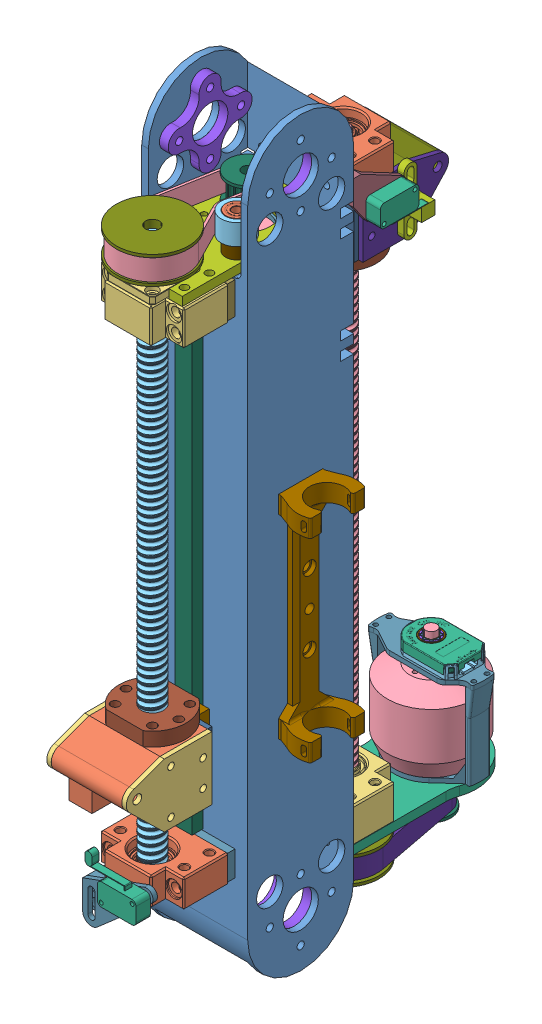
SolidWorks assembly Shoulder, configuration Default. Lengths in mm.
Overall size (114.36 533.4 280.38).
87 component instances, 45 part files, 83 mates.
Components (placement in the parent):
- Box-1: Box [Round] at origin size (76.2 533.4 76.2)
- BF12-1: BF12 [Default] at (0 614.1315 -46.7041) x (1 0 0) z (0 1 0) size (60 43 20)
- BK12-1: BK12 [Default] at (0 212.1315 -46.7041) x (-1 0 0) z (0 -1 0) size (60 46.94 35.34)
- SFU1605-450-1: SFU1605-450 [1605-400] at (0 171.1315 -71.7041) x (1 0 0) z (0 -1 0) size (16.52 16.22 450)
- BK12-2: BK12 [Default] at (0 582.269 40.2909) x (-1 0 0) z (0 1 0) size (60 46.94 35.34)
- BF12-2: BF12 [Default] at (0 230.269 40.2909) x (-1 0 0) z (0 1 0) size (60 43 20)
- SFU1605-400-3: SFU1605-400 [1605-400] at (0 623.269 65.2909) x (-1 0 0) z (0 1 0) size (16.52 16.22 400)
- J3Plate^Shoulder-1: J3Plate^Shoulder [Default] at origin size (65 6.35 120.35) (virtual)
- J2Plate^Shoulder-1: J2Plate^Shoulder [Default] at origin size (65 6.35 107.35) (virtual)
- J3MGN12R-1: J3MGN12R [Default] at origin size (12 379.5 8)
- J3MGN12C-1: J3MGN12C [Default] at (0 580.7871 -49.3066) x (1 0 0) z (0 1 0) size (27 10 45.5)
- CarriagePlate^Shoulder-1: CarriagePlate^Shoulder [Default] at (0 214.8102 -3.2066) size (50.8 45.5 3.17) (virtual)
- nut-1: nut [Default] at (0 558.0371 -71.7041) x (-1 0 0) z (0 -1 0) size (48 40 42)
- BKSpacer^Shoulder-1: BKSpacer^Shoulder [Default] at origin size (58 23 8.6) (virtual)
- BKSpacer^Shoulder-2: BKSpacer^Shoulder [Default] at (0 370.1375 81.5975) size (58 23 8.6) (virtual)
- BFSpacer^Shoulder-1: BFSpacer^Shoulder [Default] at origin size (67.1 32.07 40.22) (virtual)
- BFSpacerWSwitchMount^Shoulder-1: BFSpacerWSwitchMount^Shoulder [Default] at (0 -383.8625 81.5975) size (58 48.16 51.57) (virtual)
- J2MGN12R^Shoulder-1: J2MGN12R^Shoulder [Default] at origin size (12 329.5 8) (virtual)
- J3Adapter^Shoulder-2: J3Adapter^Shoulder [Default] at (0 224.1764 -3.2066) size (57.15 45.5 61.61) (virtual)
  - Body^J3Adapter_Shoulder-1: Body^J3Adapter_Shoulder [Default] at (38.1 26.927 0) x (0 0 -1) z (1 0 0) size (61.61 45.5 50.8) (virtual)
  - SidePlate^J3Adapter_Shoulder-1: SidePlate^J3Adapter_Shoulder [Default] at origin size (3.18 45.5 61.61) (virtual)
  - SidePlate^J3Adapter_Shoulder-2: SidePlate^J3Adapter_Shoulder [Default] at (53.975 0 0) size (3.18 45.5 61.61) (virtual)
  - 94459A340_BRASS HEAT-SET INSERT FOR PLASTIC-1: 94459A340_BRASS HEAT-SET INSERT FOR PLASTIC [94459A340] at (-18.415 340.7357 -83.735) x (0 -1 0) z (0 0 -1) size (7.22 6.55 7.22)
  - 94459A180_BRASS HEAT-SET INSERT FOR PLASTIC-1: 94459A180_BRASS HEAT-SET INSERT FOR PLASTIC [94459A180] at (13.435 343.3607 -81.9325) x (-0.837169 0 -0.546944) z (-0.546944 0 0.837169) size (7.17 9.73 7.17)
- J3MGN12C-2: J3MGN12C [Default] at (0 297.5146 42.8934) x (-1 0 0) z (0 1 0) size (27 10 45.5)
- nut-2: nut [Default] at (0 320.2646 65.2909) x (1 0 0) z (0 1 0) size (48 40 42)
- J2Adapter^Shoulder-1: J2Adapter^Shoulder [Default] at (0 654.1252 -3.2066) x (1 0 0) z (0 0 -1) size (57.15 45.5 61.61) (virtual)
  - Body^J2Adapter_Shoulder-1: Body^J2Adapter_Shoulder [Default] at (38.1 26.927 0) x (0 0 -1) z (1 0 0) size (61.61 45.5 50.8) (virtual)
  - SidePlate1fix-1: SidePlate1fix [Default] at origin size (3.18 45.5 61.61)
  - SidePlate1fix-2: SidePlate1fix [Default] at (53.975 0 0) size (3.18 45.5 61.61)
  - 94459A340_BRASS HEAT-SET INSERT FOR PLASTIC-1: 94459A340_BRASS HEAT-SET INSERT FOR PLASTIC [94459A340] at (-18.415 340.7357 -83.735) x (0 -1 0) z (0 0 -1) size (7.22 6.55 7.22)
  - 94459A180_BRASS HEAT-SET INSERT FOR PLASTIC-1: 94459A180_BRASS HEAT-SET INSERT FOR PLASTIC [94459A180] at (13.435 343.3607 -81.9325) x (-0.837169 0 -0.546944) z (-0.546944 0 0.837169) size (7.17 9.73 7.17)
- CarriagePlate^Shoulder-2: CarriagePlate^Shoulder [Default] at (0 -68.4623 -3.2066) x (-1 0 0) z (0 0 -1) size (50.8 45.5 3.17) (virtual)
- 192kvMotorEncoded-1: 192kvMotorEncoded [Default] at (0 202.8065 -135.2041) x (0 0 -1) z (1 0 0) size (63 104.52 76.93)
  - BetterKEDA-1: BetterKEDA [Default] at origin size (63 104.52 63)
  - CUI_DEVICES_AMT102-0048-N2000-S-1: CUI_DEVICES_AMT102-0048-N2000-S [Default] at (0 65.12 0) x (1 0 0) z (0 1 0) size (36.33 46.21 9.2)
    - CUI_DEVICES_AMT102-0048-N2000-S.step-1: CUI_DEVICES_AMT102-0048-N2000-S.step [Default] at origin size (36.33 46.21 9.2)
      - AMT-102-Base-REV-K.step-1: AMT-102-Base-REV-K.step [Default] x (-1 0 0) z (0 0 -1) size (28.78 43.39 9.06)
      - AMT-102-Top-Cover-REV-H.step-1: AMT-102-Top-Cover-REV-H.step [Default] at (0 0 5.23) x (-1 0 0) z (0 0 -1) size (28.6 43.26 6.55)
      - AMT-Sleeve-REV-D_ 2 mm.step-1: AMT-Sleeve-REV-D_ 2 mm.step [Default] at (0 0 -2.42) x (0.999996 0.002864 0) z (0 0 1) size (10.79 10.79 7.8)
      - AMT-Hub-Top-REV-D1.step-1: AMT-Hub-Top-REV-D1.step [Default] at (0 0 2.13) x (0.999996 0.002864 0) z (0 0 1) size (14 14 5.67)
      - AMT-Hub-Bottom-REV-B.step-1: AMT-Hub-Bottom-REV-B.step [Default] at (0 0 2.43) x (0.999998 -0.001942 0) z (0 0 1) size (17.3 17.3 3.2)
      - AMT10X-Shaft-Adaptor-REV-E.step-1: AMT10X-Shaft-Adaptor-REV-E.step [Default] at (0 0 0.03) x (0.999996 0.002864 0) z (0 0 1) size (11.8 11.8 7.8)
      - Receiver-board.step-1: Receiver-board.step [Default] at (72.2834 -20.351 3.03) x (-1 0 0) z (0 0 -1) size (26.5 26.62 0.41)
      - Rotor-board-REV F.step-1: Rotor-board-REV F.step [Default] at (0 0 2.13) x (0.807874 -0.589355 0) z (0 0 1) size (26 26 0.3)
      - Transmitter-board AMT10_AMT-102.step-1: Transmitter-board AMT10_AMT-102.step [Default] at (19.1596 -17.1102 1.22) x (-1 0 0) z (0 0 -1) size (26.63 38.43 4.41)
  - Body^192kvMotorEncoded-1: Body^192kvMotorEncoded [Default] at origin size (53 64.53 76.93) (virtual)
- 192kvMotorEncoded-2: 192kvMotorEncoded [Default] at (0 591.594 -3.2066) x (-0.707107 0 -0.707107) z (-0.707107 0 0.707107) size (63 104.52 76.93)
  - BetterKEDA-1: BetterKEDA [Default] at origin size (63 104.52 63)
  - CUI_DEVICES_AMT102-0048-N2000-S-1: CUI_DEVICES_AMT102-0048-N2000-S [Default] at (0 65.12 0) x (1 0 0) z (0 1 0) size (36.33 46.21 9.2)
    - CUI_DEVICES_AMT102-0048-N2000-S.step-1: CUI_DEVICES_AMT102-0048-N2000-S.step [Default] at origin size (36.33 46.21 9.2)
      - AMT-102-Base-REV-K.step-1: AMT-102-Base-REV-K.step [Default] x (-1 0 0) z (0 0 -1) size (28.78 43.39 9.06)
      - AMT-102-Top-Cover-REV-H.step-1: AMT-102-Top-Cover-REV-H.step [Default] at (0 0 5.23) x (-1 0 0) z (0 0 -1) size (28.6 43.26 6.55)
      - AMT-Sleeve-REV-D_ 2 mm.step-1: AMT-Sleeve-REV-D_ 2 mm.step [Default] at (0 0 -2.42) x (0.999996 0.002864 0) z (0 0 1) size (10.79 10.79 7.8)
      - AMT-Hub-Top-REV-D1.step-1: AMT-Hub-Top-REV-D1.step [Default] at (0 0 2.13) x (0.999996 0.002864 0) z (0 0 1) size (14 14 5.67)
      - AMT-Hub-Bottom-REV-B.step-1: AMT-Hub-Bottom-REV-B.step [Default] at (0 0 2.43) x (0.999998 -0.001942 0) z (0 0 1) size (17.3 17.3 3.2)
      - AMT10X-Shaft-Adaptor-REV-E.step-1: AMT10X-Shaft-Adaptor-REV-E.step [Default] at (0 0 0.03) x (0.999996 0.002864 0) z (0 0 1) size (11.8 11.8 7.8)
      - Receiver-board.step-1: Receiver-board.step [Default] at (72.2834 -20.351 3.03) x (-1 0 0) z (0 0 -1) size (26.5 26.62 0.41)
      - Rotor-board-REV F.step-1: Rotor-board-REV F.step [Default] at (0 0 2.13) x (0.807874 -0.589355 0) z (0 0 1) size (26 26 0.3)
      - Transmitter-board AMT10_AMT-102.step-1: Transmitter-board AMT10_AMT-102.step [Default] at (19.1596 -17.1102 1.22) x (-1 0 0) z (0 0 -1) size (26.63 38.43 4.41)
  - Body^192kvMotorEncoded-1: Body^192kvMotorEncoded [Default] at origin size (53 64.53 76.93) (virtual)
- 15Tpulley-3: 15Tpulley [Default] at (0 175.8815 -135.2041) size (28 28 28)
- 15Tpulley-4: 15Tpulley [Default] at (0 618.519 -3.2066) x (-1 0 0) z (0 0 1) size (28 28 28)
- 30Tpulley-3: 30Tpulley [Default] at (0 618.519 65.2909) size (52 20 52)
- 30Tpulley-4: 30Tpulley [Default] at (0 175.8815 -71.7041) size (52 20 52)
- J3Belt51T^Shoulder-1: J3Belt51T^Shoulder [Default] at origin size (49.49 15 101.05) (virtual)
- TensionPillarJ3-1: TensionPillarJ3 [Default] at (-42.5291 257.8915 3.8215) size (33.31 25.73 33.31)
  - 92510A774_ALUM UNTHRD SPACER-1-1: 92510A774_ALUM UNTHRD SPACER-1 [92510A774] at (20.3041 -69.3725 -110.4505) x (1 0 0) z (0 1 0) size (15.88 15.88 9.53)
  - 98019A228_MIL SPEC. 300 SERIES SS FLAT WASHER-1: 98019A228_MIL SPEC. 300 SERIES SS FLAT WASHER [98019A228] at (20.3041 -74.8462 -110.4505) x (0.972939 0 -0.231063) z (0.231063 0 0.972939) size (9.53 0.71 9.53)
  - 60355K701_BALL BEARING-1: 60355K701_BALL BEARING [60355K701] at (20.3041 -77.3354 -110.4505) x (1 0 0) z (0 1 0) size (15.88 15.88 4.98)
  - Roller^TensionPillarJ3-1: Roller^TensionPillarJ3 [Default] at (-2.0675 -22.8548 2.6827) size (33.31 15 33.31) (virtual)
  - 60355K701_BALL BEARING-2: 60355K701_BALL BEARING [60355K701] at (20.3041 -87.8548 -110.4505) x (1 0 0) z (0 1 0) size (15.88 15.88 4.98)
- J2Belt52T^Shoulder-1: J2Belt52T^Shoulder [Default] at origin size (49.49 15 106.05) (virtual)
- TensionPillarJ2-1: TensionPillarJ2 [Default] at (19.05 605.8815 23.7809) x (-1 0 0) z (0 1 0) size (22.23 22.23 25.73)
  - 92510A774_ALUM UNTHRD SPACER-1-1: 92510A774_ALUM UNTHRD SPACER-1 [92510A774] x (1 0 0) z (0 0 -1) size (15.88 15.88 9.53)
  - 98019A228_MIL SPEC. 300 SERIES SS FLAT WASHER-1: 98019A228_MIL SPEC. 300 SERIES SS FLAT WASHER [98019A228] at (0 0 5.4737) x (0.972939 -0.231063 0) z (0.231063 0.972939 0) size (9.53 0.71 9.53)
  - 60355K701_BALL BEARING-1: 60355K701_BALL BEARING [60355K701] at (0 0 7.9629) x (1 0 0) z (0 0 -1) size (15.88 15.88 4.98)
  - Roller^TensionPillarJ2-1: Roller^TensionPillarJ2 [Default] at (-22.3716 113.1333 -52.2073) x (1 0 0) z (0 1 0) size (22.23 15 22.23) (virtual)
  - 60355K701_BALL BEARING-2: 60355K701_BALL BEARING [60355K701] at (0 0 18.4823) x (1 0 0) z (0 0 -1) size (15.88 15.88 4.98)
- switch-1: switch [Default] at (43.25 594.2315 -52.9416) x (0 0 1) z (0 1 0) size (39.3 10.3 27.5)
- Trigger^Shoulder-1: Trigger^Shoulder [Default] at (-1.6066 -39.0023 -12.3199) size (17.46 47.62 9.53) (virtual)
- switch-2: switch [Default] at (16.85 229.869 91.6159) x (1 0 0) z (0 -1 0) size (39.3 10.3 27.5)
- ShaftSupp^Shoulder-1: ShaftSupp^Shoulder [Default] at origin size (6.35 60.32 60.32)
- ShaftSupp^Shoulder-2: ShaftSupp^Shoulder [Default] at (0 457.2 0) size (6.35 60.32 60.32)
- ShaftSupp^Shoulder-5: ShaftSupp^Shoulder [Default] at (0 0 -6.4131) x (-1 0 0) z (0 0 -1) size (6.35 60.32 60.32)
- ShaftSupp^Shoulder-6: ShaftSupp^Shoulder [Default] at (0 457.2 -6.4131) x (-1 0 0) z (0 0 -1) size (6.35 60.32 60.32)
- WireGuide^Shoulder-1: WireGuide^Shoulder [Default] at origin size (26.79 152.4 42.24) (virtual)
Mates (geometry in assembly coordinates):
- Parallel1: parallel anti-aligned: plane of Box-1 through (-33.3375 186.9315 -41.3066) normal (0 0 -1); plane of BF12-1 through (29 605.1315 -46.7041) normal (0 0 1)
- Width1: width anti-aligned: plane of BF12-1 through (30 605.1315 -78.2041) normal (1 0 0); plane of BF12-1 through (-30 605.1315 -47.7041) normal (-1 0 0); plane of Box-1 through (38.1 644.1315 -3.2066) normal (1 0 0); plane of Box-1 through (-38.1 186.9315 -3.2066) normal (-1 0 0)
- Distance6: distance anti-aligned: plane of Box-1 through (-33.3375 186.9315 -41.3066) normal (0 0 -1); plane of BK12-1 through (-29 223.6315 -46.7041) normal (0 0 1)
- Width2: width aligned: plane of BK12-1 through (30 223.6315 -47.7041) normal (1 0 0); plane of BK12-1 through (-30 223.6315 -78.2041) normal (-1 0 0); plane of Box-1 through (-38.1 186.9315 -3.2066) normal (-1 0 0); plane of Box-1 through (38.1 644.1315 -3.2066) normal (1 0 0)
- Parallel3: parallel aligned: plane of BK12-1 through (29 224.6315 -47.7041) normal (0 1 0)
- Coincident11: coincident: line of SFU1605-450-1 through (0 185.8815 -71.7041) axis (0 -1 0)
- Concentric6: concentric anti-aligned: cylinder of BK12-1 through (0 220.1315 -71.7041) axis (0 1 0) radius 6; cylinder of SFU1605-450-1 through (0 186.1315 -71.7041) axis (0 -1 0) radius 5
- Coincident12: coincident anti-aligned: plane of BK12-1 through (7.2358 225.1315 -64.4683) normal (0 1 0); plane of SFU1605-450-1 through (0 225.1315 -71.7041) normal (0 -1 0)
- Coincident13: coincident anti-aligned: plane of BF12-1 through (-6.5021 610.1315 -65.202) normal (0 -1 0); plane of SFU1605-450-1 through (0 610.1315 -71.7041) normal (0 1 0)
- Distance3: distance = 12.7 mm: plane of BK12-1 through (29 199.6315 -47.7041) normal (0 -1 0); line of Box-1 through (38.1 186.9315 -41.3066) axis (-1 0 0)
- Coincident27: coincident: line of SFU1605-400-3 through (0 608.519 65.2909) axis (0 1 0)
- Concentric18: concentric anti-aligned: cylinder of BK12-2 through (0 582.269 65.2909) axis (0 -1 0) radius 6; cylinder of SFU1605-400-3 through (0 608.269 65.2909) axis (0 1 0) radius 5
- Distance8: distance anti-aligned: plane of Box-1 through (-33.3375 186.9315 34.8934) normal (0 0 1); plane of BK12-2 through (-29 570.769 40.2909) normal (0 0 -1)
- Coincident29: coincident anti-aligned: plane of BK12-2 through (7.2358 569.269 58.0551) normal (0 -1 0); plane of SFU1605-400-3 through (0 569.269 65.2909) normal (0 1 0)
- Coincident30: coincident anti-aligned: plane of BF12-2 through (-6.5021 234.269 58.7888) normal (0 1 0); plane of SFU1605-400-3 through (0 234.269 65.2909) normal (0 -1 0)
- Concentric19: concentric anti-aligned: cylinder of BF12-2 through (0 227.069 65.2909) axis (0 1 0) radius 5; cylinder of SFU1605-400-3 through (0 234.269 65.2909) axis (0 -1 0) radius 5
- Distance5: distance = 33.3375 mm: line of Box-1 through (38.1 186.9315 34.8934) axis (-1 0 0); plane of BF12-2 through (29 220.269 41.2909) normal (0 -1 0)
- Coincident35: coincident anti-aligned: plane of J3MGN12R-1 through (0 0 -49.3066) normal (0 0 -1); plane of J3MGN12C-1 through (-6 603.5371 -49.3066) normal (0 0 1)
- Width3: width anti-aligned: plane of J3MGN12C-1 through (13.5 603.5371 -44.3066) normal (1 0 0); plane of J3MGN12R-1 through (-13.5 603.5371 -44.3066) normal (-1 0 0); plane of J3MGN12C-1 through (-6 604.1315 -49.3066) normal (-1 0 0); plane of J3MGN12R-1 through (6 604.1315 -49.3066) normal (1 0 0)
- Coincident36: coincident anti-aligned: plane of J3MGN12C-1 through (13.5 603.5371 -54.3066) normal (0 0 -1); plane of CarriagePlate^Shoulder-1 through (0 214.8102 -54.3066) normal (0 0 1)
- Concentric22: concentric anti-aligned: cylinder of J3MGN12C-1 through (10 590.7871 -50.3066) axis (0 0 -1) radius 1.5; cylinder of CarriagePlate^Shoulder-1 through (10 590.7871 -57.4816) axis (0 0 1) radius 1.5
- Concentric23: concentric anti-aligned: cylinder of J3MGN12C-1 through (-10 570.7871 -50.3066) axis (0 0 -1) radius 1.5; cylinder of CarriagePlate^Shoulder-1 through (-10 570.7871 -57.4816) axis (0 0 1) radius 1.5
- Concentric24: concentric aligned: cylinder of SFU1605-450-1 through (0 610.1315 -71.7041) axis (0 1 0) radius 5; cylinder of nut-1 through (0 548.0371 -71.7041) axis (0 1 0) radius 8
- Concentric25: concentric aligned: cylinder of BF12-1 through (0 610.9315 -71.7041) axis (0 1 0) radius 5; cylinder of SFU1605-450-1 through (0 610.1315 -71.7041) axis (0 1 0) radius 5
- Coincident37: coincident anti-aligned: plane of CarriagePlate^Shoulder-1 through (-25.4 558.0371 -57.4816) normal (0 -1 0); plane of nut-1 through (0 558.0371 -71.7041) normal (0 1 0)
- Parallel4: parallel anti-aligned: plane of Box-1 through (-33.3375 186.9315 34.8934) normal (0 0 1); plane of BF12-2 through (-29 221.269 40.2909) normal (0 0 -1)
- Concentric27: concentric anti-aligned: cylinder of BK12-2 through (-23 575.769 40.2909) axis (0 0 1) radius 3.3; cylinder of BKSpacer^Shoulder-2 through (-23 575.769 102.6848) axis (0 0 -1) radius 3.3
- Concentric28: concentric anti-aligned: cylinder of BK12-2 through (23 575.769 40.2909) axis (0 0 1) radius 3.3; cylinder of BKSpacer^Shoulder-2 through (23 575.769 102.6848) axis (0 0 -1) radius 3.3
- Coincident42: coincident anti-aligned: plane of Box-1 through (-33.3375 186.9315 34.8934) normal (0 0 1); plane of BKSpacer^Shoulder-2 through (0 370.1375 34.8934) normal (0 0 -1)
- Concentric29: concentric anti-aligned: cylinder of BF12-2 through (23 230.269 40.2909) axis (0 0 1) radius 3.3; cylinder of BFSpacerWSwitchMount^Shoulder-1 through (23 230.269 101.0198) axis (0 0 -1) radius 3.3
- Concentric30: concentric anti-aligned: cylinder of BF12-2 through (-23 230.269 40.2909) axis (0 0 1) radius 3.3; cylinder of BFSpacerWSwitchMount^Shoulder-1 through (-23 230.269 101.0198) axis (0 0 -1) radius 3.3
- Coincident43: coincident anti-aligned: plane of Box-1 through (-33.3375 186.9315 34.8934) normal (0 0 1); plane of BFSpacerWSwitchMount^Shoulder-1 through (0 -383.8625 34.8934) normal (0 0 -1)
- Concentric32: concentric anti-aligned: cylinder of nut-1 through (0 590.0371 -71.7041) axis (0 -1 0) radius 14; cylinder of J3Adapter^Shoulder-2/Body^J3Adapter_Shoulder-1 through (0 496.785 -71.7041) axis (0 1 0) radius 14.635
- Parallel6: parallel anti-aligned: plane of CarriagePlate^Shoulder-1 through (0 214.8102 -57.4816) normal (0 0 -1); plane of J3Adapter^Shoulder-2/Body^J3Adapter_Shoulder-1 through (38.1 496.785 -57.4816) normal (0 0 1)
- Coincident47: coincident anti-aligned: plane of nut-1 through (0 558.0371 -71.7041) normal (0 1 0); plane of J3Adapter^Shoulder-2/Body^J3Adapter_Shoulder-1 through (-25.4 558.0371 -57.4816) normal (0 -1 0)
- Coincident48: coincident anti-aligned: plane of nut-1 through (0 558.0371 -71.7041) normal (0 1 0); plane of J3Adapter^Shoulder-2/Body^J3Adapter_Shoulder-1 through (-25.4 558.0371 -57.4816) normal (0 -1 0)
- Coincident49: coincident anti-aligned: plane of nut-1 through (0 558.0371 -71.7041) normal (0 1 0); plane of J3Adapter^Shoulder-2/Body^J3Adapter_Shoulder-1 through (-25.4 558.0371 -57.4816) normal (0 -1 0)
- Coincident51: coincident anti-aligned: plane of J2MGN12R^Shoulder-1 through (0 0 42.8934) normal (0 0 1); plane of J3MGN12C-2 through (6 320.2646 42.8934) normal (0 0 -1)
- Width6: width anti-aligned: plane of J3MGN12C-2 through (-13.5 320.2646 37.8934) normal (-1 0 0); plane of J2MGN12R^Shoulder-1 through (13.5 320.2646 37.8934) normal (1 0 0); plane of J3MGN12C-2 through (6 569.769 42.8934) normal (1 0 0); plane of J2MGN12R^Shoulder-1 through (-6 569.769 42.8934) normal (-1 0 0)
- Concentric34: concentric anti-aligned: cylinder of SFU1605-400-3 through (0 608.269 65.2909) axis (0 1 0) radius 5; cylinder of nut-2 through (0 330.2646 65.2909) axis (0 -1 0) radius 8
- Coincident52: coincident anti-aligned: plane of J3MGN12C-2 through (0 320.2646 42.8934) normal (0 1 0); plane of nut-2 through (0 320.2646 65.2909) normal (0 -1 0)
- Concentric35: concentric anti-aligned: cylinder of nut-2 through (0 288.2646 65.2909) axis (0 1 0) radius 14; cylinder of J2Adapter^Shoulder-1/Body^J2Adapter_Shoulder-1 through (0 381.5167 65.2909) axis (0 -1 0) radius 14.635
- Parallel7: parallel anti-aligned: plane of J3MGN12C-2 through (-13.5 320.2646 47.8934) normal (0 0 1); plane of J2Adapter^Shoulder-1/Body^J2Adapter_Shoulder-1 through (38.1 381.5167 51.0684) normal (0 0 -1)
- Coincident54: coincident anti-aligned: plane of nut-2 through (0 320.2646 65.2909) normal (0 -1 0); plane of J2Adapter^Shoulder-1/Body^J2Adapter_Shoulder-1 through (-25.4 320.2646 51.0684) normal (0 1 0)
- Concentric36: concentric anti-aligned: cylinder of J3MGN12C-2 through (10 307.5146 43.8934) axis (0 0 1) radius 1.5; cylinder of CarriagePlate^Shoulder-2 through (10 307.5146 51.0684) axis (0 0 -1) radius 1.5
- Concentric37: concentric anti-aligned: cylinder of J3MGN12C-2 through (-10 287.5146 43.8934) axis (0 0 1) radius 1.5; cylinder of CarriagePlate^Shoulder-2 through (-10 287.5146 51.0684) axis (0 0 -1) radius 1.5
- Coincident55: coincident anti-aligned: plane of J3MGN12C-2 through (-13.5 320.2646 47.8934) normal (0 0 1); plane of CarriagePlate^Shoulder-2 through (0 -68.4623 47.8934) normal (0 0 -1)
- Parallel8: parallel aligned: plane of BF12-2 through (29 240.269 41.2909) normal (0 1 0)
- Concentric38: concentric aligned: cylinder of J3Plate^Shoulder-1 through (0 193.2815 -135.2041) axis (0 1 0) radius 15.875; cylinder of 192kvMotorEncoded-1/BetterKEDA-1 through (0 173.2815 -135.2041) axis (0 1 0) radius 4
- Concentric39: concentric aligned: cylinder of J3Plate^Shoulder-1 through (0 193.2815 -113.0041) axis (0 1 0) radius 2; cylinder of 192kvMotorEncoded-1/Body^192kvMotorEncoded-1 through (0 199.6315 -113.0041) axis (0 1 0) radius 2
- Coincident56: coincident anti-aligned: plane of J3Plate^Shoulder-1 through (54.75 199.6315 -116.3667) normal (0 1 0); plane of 192kvMotorEncoded-1/Body^192kvMotorEncoded-1 through (0 199.6315 -135.2041) normal (0 -1 0)
- Concentric40: concentric aligned: cylinder of J2Plate^Shoulder-1 through (0 601.119 -3.2066) axis (0 -1 0) radius 15.875; cylinder of 192kvMotorEncoded-2/BetterKEDA-1 through (0 621.119 -3.2066) axis (0 -1 0) radius 4
- Concentric41: concentric aligned: cylinder of J2Plate^Shoulder-1 through (-15.6978 601.119 12.4912) axis (0 -1 0) radius 2; cylinder of 192kvMotorEncoded-2/Body^192kvMotorEncoded-1 through (-15.6978 594.769 12.4912) axis (0 -1 0) radius 2
- Coincident57: coincident anti-aligned: plane of J2Plate^Shoulder-1 through (0 594.769 0) normal (0 -1 0); plane of 192kvMotorEncoded-2/Body^192kvMotorEncoded-1 through (0 594.769 -3.2066) normal (0 1 0)
- Concentric42: concentric anti-aligned: cylinder of 192kvMotorEncoded-1/BetterKEDA-1 through (0 173.2815 -135.2041) axis (0 1 0) radius 4; cylinder of 15Tpulley-3 through (0 183.8815 -135.2041) axis (0 -1 0) radius 4
- Concentric44: concentric anti-aligned: cylinder of 192kvMotorEncoded-2/BetterKEDA-1 through (0 621.119 -3.2066) axis (0 -1 0) radius 4; cylinder of 15Tpulley-4 through (0 610.519 -3.2066) axis (0 1 0) radius 4
- Concentric45: concentric anti-aligned: cylinder of SFU1605-400-3 through (0 608.269 65.2909) axis (0 1 0) radius 5; cylinder of 30Tpulley-3 through (0 626.519 65.2909) axis (0 -1 0) radius 5
- Coincident61: coincident anti-aligned: circle of SFU1605-400-3; plane of 30Tpulley-3 through (0 608.519 65.2909) normal (0 -1 0)
- Coincident62: coincident aligned: plane of 15Tpulley-4 through (0 626.519 -3.2066) normal (0 -1 0); plane of 30Tpulley-3 through (0 626.519 65.2909) normal (0 -1 0)
- Concentric47: concentric aligned: cylinder of SFU1605-450-1 through (0 186.1315 -71.7041) axis (0 -1 0) radius 5; cylinder of 30Tpulley-4 through (0 183.8815 -71.7041) axis (0 -1 0) radius 5
- Coincident63: coincident anti-aligned: circle of SFU1605-450-1; plane of 30Tpulley-4 through (0 185.8815 -71.7041) normal (0 1 0)
- Coincident64: coincident aligned: plane of 15Tpulley-3 through (0 167.8815 -135.2041) normal (0 1 0); plane of 30Tpulley-4 through (0 167.8815 -71.7041) normal (0 1 0)
- Concentric48: concentric aligned: cylinder of J3Plate^Shoulder-1 through (-22.225 199.6315 -106.6291) axis (0 -1 0) radius 2.6035; cylinder of TensionPillarJ3-1/92510A774_ALUM UNTHRD SPACER-1-1 through (-22.225 193.2815 -106.6291) axis (0 -1 0) radius 3.2004
- Coincident65: coincident anti-aligned: plane of J3Plate^Shoulder-1 through (54.75 193.2815 -116.3667) normal (0 -1 0); plane of TensionPillarJ3-1/92510A774_ALUM UNTHRD SPACER-1-1 through (-22.225 193.2815 -106.6291) normal (0 1 0)
- Concentric49: concentric aligned: cylinder of J2Plate^Shoulder-1 through (19.05 587.4052 23.7809) axis (0 1 0) radius 2.6035; cylinder of TensionPillarJ2-1/92510A774_ALUM UNTHRD SPACER-1-1 through (19.05 601.119 23.7809) axis (0 1 0) radius 3.2004
- Coincident66: coincident anti-aligned: plane of J2Plate^Shoulder-1 through (0 601.119 0) normal (0 1 0); plane of TensionPillarJ2-1/92510A774_ALUM UNTHRD SPACER-1-1 through (19.05 601.119 23.7809) normal (0 -1 0)
- Parallel9: parallel anti-aligned: plane of Box-1 through (38.1 644.1315 -3.2066) normal (1 0 0); plane of switch-1 through (38.1 594.2315 -52.9416) normal (-1 0 0)
- Distance9: distance = 12.7 mm aligned: plane of switch-1 through (48.4 591.4315 -52.9416) normal (0 -1 0); plane of BF12-1 through (-29 604.1315 -47.7041) normal (0 -1 0)
- LimitDistance1: limit distance = 0.5945 mm anti-aligned: plane of J3Adapter^Shoulder-2/Body^J3Adapter_Shoulder-1 through (38.1 603.5371 -3.2066) normal (0 1 0); plane of BF12-1 through (-29 604.1315 -47.7041) normal (0 -1 0)
- LimitDistance2: limit distance = 323.4055 mm anti-aligned: plane of nut-1 through (0 548.0371 -71.7041) normal (0 -1 0); plane of BK12-1 through (29 224.6315 -47.7041) normal (0 1 0)
- Coincident71: coincident: line of switch-1 through (45.75 586.3315 -86.9416) axis (-1 0 0); plane of Trigger^Shoulder-1 through (-1.6066 -39.0023 -86.9416) normal (0 0 -1)
- LimitDistance3: limit distance = 239.5045 mm anti-aligned: plane of nut-2 through (0 330.2646 65.2909) normal (0 1 0); plane of BK12-2 through (29 569.769 41.2909) normal (0 -1 0)
- LimitDistance4: limit distance = 34.4955 mm anti-aligned: plane of J2Adapter^Shoulder-1/Body^J2Adapter_Shoulder-1 through (38.1 274.7646 -3.2066) normal (0 -1 0); plane of BF12-2 through (29 240.269 41.2909) normal (0 1 0)
- Parallel10: parallel anti-aligned: plane of BF12-2 through (16 221.269 83.2909) normal (0 0 1); plane of switch-2 through (16.85 229.869 86.4659) normal (0 0 -1)
- Coincident76: coincident aligned: plane of switch-2 through (0 229.869 91.6159) normal (1 0 0)
- Tangent1: tangent aligned: plane of BF12-2 through (29 240.269 41.2909) normal (0 1 0); cylinder of switch-2 through (-17.15 237.769 94.1159) axis (0 0 -1) radius 2.5
- Coincident79: coincident anti-aligned: plane of BFSpacerWSwitchMount^Shoulder-1 through (0 -383.8625 86.4659) normal (0 0 1); plane of switch-2 through (16.85 229.869 86.4659) normal (0 0 -1)
- Concentric52: concentric aligned: cylinder of Box-1 through (33.3375 644.1315 -3.2066) axis (1 0 0) radius 12.7; cylinder of ShaftSupp^Shoulder-2 through (26.9875 644.1315 -3.2066) axis (1 0 0) radius 12.7
- Coincident80: coincident anti-aligned: plane of Box-1 through (33.3375 644.1315 -3.2066) normal (-1 0 0); plane of ShaftSupp^Shoulder-2 through (33.3375 654.4171 18.1915) normal (1 0 0)
- Parallel11: parallel aligned: plane of ShaftSupp^Shoulder-1 through (0 0 0) normal (0 1 0); plane of ShaftSupp^Shoulder-2 through (0 457.2 0) normal (0 1 0)
- Coincident81: coincident anti-aligned: plane of BFSpacer^Shoulder-1 through (38.1 605.1315 28.1658) normal (1 0 0); plane of switch-1 through (38.1 594.2315 -52.9416) normal (-1 0 0)
- Coincident83: coincident anti-aligned: plane of J3Adapter^Shoulder-2/SidePlate^J3Adapter_Shoulder-2 through (28.575 590.8371 -111.1566) normal (1 0 0); plane of Trigger^Shoulder-1 through (28.575 -39.0023 -12.3199) normal (-1 0 0)
- Concentric58: concentric anti-aligned: cylinder of J3Adapter^Shoulder-2/SidePlate^J3Adapter_Shoulder-2 through (25.4 564.9121 -86.9416) axis (1 0 0) radius 2.3813; cylinder of Trigger^Shoulder-1 through (33.3375 564.9121 -86.9416) axis (-1 0 0) radius 2.3813
